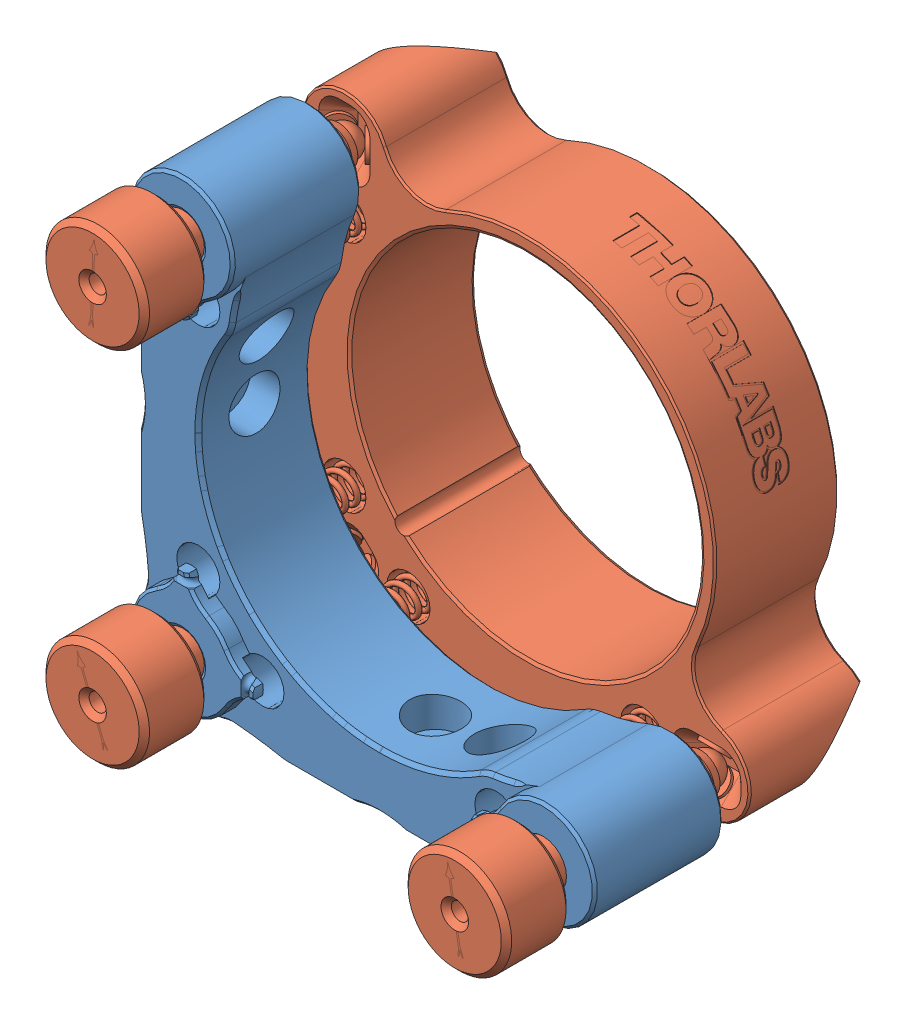
SolidWorks assembly POLARIS-K2T, configuration Default. Lengths in mm.
Overall size (70.19 70.19 56.2).
2 component instances, 2 part files, 6 mates.
Components (placement in the parent):
- POLARIS-K2T_base_plate-1: POLARIS-K2T_base_plate [Default] at (-35.7609 -40.1333 -48.0572) size (70.19 70.19 19.14)
- POLARIS-K2T_front_plate-1: POLARIS-K2T_front_plate [Default] at (-35.7609 -40.1333 -49.8822) size (68.58 68.58 56.2)
Mates (geometry in assembly coordinates):
- Coincident1: coincident aligned: plane of POLARIS-K2T_base_plate-1 through (-35.7609 -40.1333 0) normal (0 0 1); plane of assembly through (0 0 0) normal (0 0 1)
- Coincident2: coincident anti-aligned: plane of POLARIS-K2T_base_plate-1 through (-35.7609 0 -48.0572) normal (0 -1 0); plane of assembly through (0 0 0) normal (0 1 0)
- Coincident3: coincident anti-aligned: plane of POLARIS-K2T_base_plate-1 through (0 -40.1333 -48.0572) normal (-1 0 0); plane of assembly through (0 0 0) normal (1 0 0)
- Concentric1: concentric anti-aligned: cylinder of POLARIS-K2T_base_plate-1 through (0 0 10.795) axis (0 0 -1) radius 26.67; cylinder of POLARIS-K2T_front_plate-1 through (0 0 -31.67) axis (0 0 1) radius 25.8445
- Parallel1: parallel aligned: plane of POLARIS-K2T_base_plate-1 through (0 -35.56 10.795) normal (0 -1 0); plane of POLARIS-K2T_front_plate-1 through (-26.67 -33.02 -31.67) normal (0 -1 0)
- Distance2: distance = 5 mm anti-aligned: plane of POLARIS-K2T_base_plate-1 through (0 0 -8.255) normal (0 0 -1); plane of POLARIS-K2T_front_plate-1 through (-14.6486 31.144 -13.255) normal (0 0 1)
